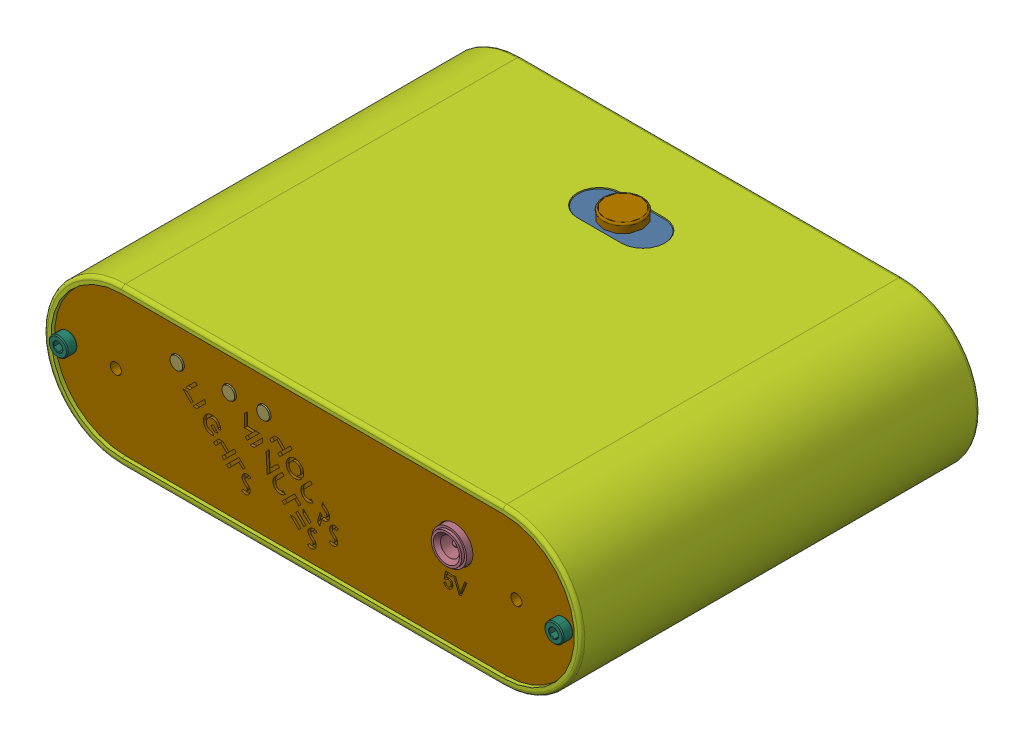
SolidWorks assembly assembly, configuration Défaut. Lengths in mm.
Overall size (155 47.3 119.91).
312 component instances, 69 part files, 68 mates.
Components (placement in the parent):
- board2-1: board2 [Défaut] at (0 -11.75 72.25) size (122.67 19.21 69.85)
  - pcb-1: pcb [Défaut] at origin size (121.6 1.5 65.9)
  - DIP18N.step-1: DIP18N.step [Défaut] at (-50.7835 3.7087 35.4382) x (0 0 1) z (-1 0 0) size (8.53 6.85 19.5)
  - DIP18N.step-2: DIP18N.step [Défaut] at (31.1067 3.7087 35.4997) x (0 0 1) z (-1 0 0) size (8.53 6.85 19.5)
  - DIP18N.step-3: DIP18N.step [Défaut] at (5.6608 3.7087 35.5611) x (0 0 1) z (-1 0 0) size (8.53 6.85 19.5)
  - DIP18N.step-4: DIP18N.step [Défaut] at (-25.3559 3.7087 35.5399) x (0 0 1) z (-1 0 0) size (8.53 6.85 19.5)
  - DIP18N.step-5: DIP18N.step [Défaut] at (-15.751 3.7087 -7.8923) x (0.008727 0 -0.999962) z (0.999962 0 0.008727) size (8.53 6.85 19.5)
  - DIP18N.step-6: DIP18N.step [Défaut] at (34.3108 3.7087 -7.8662) x (0.008727 0 -0.999962) z (0.999962 0 0.008727) size (8.53 6.85 19.5)
  - Screw Terminal Block 5mm-2: Screw Terminal Block 5mm [Valor predeterminado] at (0.4217 1.5 23.933) x (-0.999962 0 -0.008727) z (0.008727 0 -0.999962) size (10.6 16.9 9)
  - Seeeduino Xiao.step-1: Seeeduino Xiao.step [Défaut] at (-88.5187 11.44 25.9289) x (-0.008727 0 0.999962) z (-0.999962 0 -0.008727) size (17.8 4.27 22.5)
  - DS3231 RTC.step-1: DS3231 RTC.step [Défaut] at (20.896 7 25.5045) x (-1 0 0) z (0 -1 0) size (44.75 22.8 13.53)
  - zl202-8_p2-54_l10-2_w5-08_h8-89.stp-1: zl202-8_p2-54_l10-2_w5-08_h8-89.stp [Défaut] at (-55.033 1.5 3.5455) x (0 0 1) z (-1 0 0) size (10.16 11.94 5.08)
- box-1: box [Défaut] at (0 0 115) x (-1 0 0) z (0 0 -1) size (155 45 115)
- front-panel-1: front-panel [Défaut] at (0 0 10) size (150.6 40.6 3)
- back-panel-1: back-panel [Défaut] at (0 0 114) x (-1 0 0) z (0 0 -1) size (150.8 40.8 4)
- tubes-support-1: tubes-support [Défaut] at (0 0 31.6) size (147.45 40.6 8)
- beam-1: beam [Défaut] at (-60.75 -11 35) size (10.11 18.11 75.6)
- IN-12A.stp-1: IN-12A.stp [Défaut] at (-18 0 1.1) x (0 0 -1) z (-1 0 0) size (38.92 31 22.58)
  - 2.stp-1: 2.stp [Défaut] at origin size (2.7 24.17 15.83)
  - 3.stp-1: 3.stp [Défaut] at (-12.2 0 0) x (0 0 -1) z (-1 0 0) size (2 1.5 18.5)
  - 4.stp-1: 4.stp [Défaut] at (-12.2 0 0) x (0 0 1) z (-1 0 0) size (2 1.5 18.5)
  - 5.stp-1: 5.stp [Défaut] at (-12 0 0) x (0 0 -1) z (1 0 0) size (2.1 2.1 1)
  - 5.stp-2: 5.stp [Défaut] at (-10.8 0 0) x (0 0 -1) z (1 0 0) size (2.1 2.1 1)
  - 5.stp-3: 5.stp [Défaut] at (-9.6 0 0) x (0 0 -1) z (1 0 0) size (2.1 2.1 1)
  - 5.stp-4: 5.stp [Défaut] at (-8.4 0 0) x (0 0 -1) z (1 0 0) size (2.1 2.1 1)
  - 5.stp-5: 5.stp [Défaut] at (-7.2 0 0) x (0 0 -1) z (1 0 0) size (2.1 2.1 1)
  - 5.stp-6: 5.stp [Défaut] at (-6 0 0) x (0 0 -1) z (1 0 0) size (2.1 2.1 1)
  - 5.stp-7: 5.stp [Défaut] at (-4.8 0 0) x (0 0 -1) z (1 0 0) size (2.1 2.1 1)
  - 5.stp-8: 5.stp [Défaut] at (-3.6 0 0) x (0 0 -1) z (1 0 0) size (2.1 2.1 1)
  - 5.stp-9: 5.stp [Défaut] at (-2.4 0 0) x (0 0 -1) z (1 0 0) size (2.1 2.1 1)
  - 5.stp-10: 5.stp [Défaut] at (-1.2 0 0) x (0 0 -1) z (1 0 0) size (2.1 2.1 1)
  - 6.stp-1: 6.stp [Défaut] at (-11 16.1596 7.8778) x (0 -0.787778 0.61596) z (-1 0 0) size (2.1 2.1 1)
  - 7.stp-1: 7.stp [Défaut] at (-9.8 16.1596 7.8778) x (0 -0.787778 0.61596) z (-1 0 0) size (2.1 2.1 1)
  - 8.stp-1: 8.stp [Défaut] at (-8.6 16.1596 7.8778) x (0 -0.787778 0.61596) z (-1 0 0) size (2.1 2.1 1)
  - 9.stp-1: 9.stp [Défaut] at (-7.4 16.1596 7.8778) x (0 -0.787778 0.61596) z (-1 0 0) size (2.1 2.1 1)
  - 10.stp-1: 10.stp [Défaut] at (-6.2 16.1596 7.8778) x (0 -0.787778 0.61596) z (-1 0 0) size (2.1 2.1 1)
  - 11.stp-1: 11.stp [Défaut] at (-5 16.1596 7.8778) x (0 -0.787778 0.61596) z (-1 0 0) size (2.1 2.1 1)
  - 12.stp-1: 12.stp [Défaut] at (-3.8 16.1596 7.8778) x (0 -0.787778 0.61596) z (-1 0 0) size (2.1 2.1 1)
  - 13.stp-1: 13.stp [Défaut] at (-2.6 16.1596 7.8778) x (0 -0.787778 0.61596) z (-1 0 0) size (2.1 2.1 1)
  - 14.stp-1: 14.stp [Défaut] at (-1.4 16.1596 7.8778) x (0 -0.787778 0.61596) z (-1 0 0) size (2.1 2.1 1)
  - 15.stp-1: 15.stp [Défaut] at (-0.2 16.1596 7.8778) x (0 -0.787778 0.61596) z (-1 0 0) size (2.1 2.1 1)
  - 5.stp-11: 5.stp [Défaut] x (0 0 -1) z (1 0 0) size (2.1 2.1 1)
  - 5.stp-12: 5.stp [Défaut] at (-13.2 0 0) x (0 0 -1) z (1 0 0) size (2.1 2.1 1)
  - 16.stp-1: 16.stp [Défaut] at (1 16.1596 7.8778) x (0 -0.787778 0.61596) z (-1 0 0) size (2.1 2.1 1)
  - 17.stp-1: 17.stp [Défaut] at (-12.2 16.1596 7.8778) x (0 -0.787778 0.61596) z (-1 0 0) size (2.1 2.1 1)
  - 18.stp-1: 18.stp [Défaut] at (-13.2 0 0) x (0 0 -1) z (-1 0 0) size (15.83 24.17 12.28)
  - 19.stp-1: 19.stp [Défaut] x (1 0 0) z (0 1 0) size (1.51 1.46 20.68)
  - 20.stp-1: 20.stp [Défaut] at (1 0 0) size (4 22.27 2.42)
  - 21.stp-1: 21.stp [Défaut] at (-13.4 0 0) x (0 0 -1) z (-1 0 0) size (15.83 24.17 1)
  - 22.stp-1: 22.stp [Défaut] at (-14.4 0 0) x (0 0 -1) z (-1 0 0) size (15.83 27.29 2)
  - 23.stp-1: 23.stp [Défaut] x (0 0 -1) z (-1 0 0) size (21 31 33)
  - 24.stp-1: 24.stp [Défaut] x (0 0 -1) z (-1 0 0) size (1 1 15.5)
  - 24.stp-2: 24.stp [Défaut] at (0 -4.5 0) x (0 0 -1) z (-1 0 0) size (1 1 15.5)
  - 24.stp-3: 24.stp [Défaut] at (0 -8 -1.75) x (0 0 -1) z (-1 0 0) size (1 1 15.5)
  - 24.stp-4: 24.stp [Défaut] at (0 -9 -5.75) x (0 0 -1) z (-1 0 0) size (1 1 15.5)
  - 24.stp-5: 24.stp [Défaut] at (0 -8 -9.75) x (0 0 -1) z (-1 0 0) size (1 1 15.5)
  - 24.stp-6: 24.stp [Défaut] at (0 -4.5 -11.5) x (0 0 -1) z (-1 0 0) size (1 1 15.5)
  - 24.stp-7: 24.stp [Défaut] at (0 0 -11.5) x (0 0 -1) z (-1 0 0) size (1 1 15.5)
  - 24.stp-8: 24.stp [Défaut] at (0 4.5 -11.5) x (0 0 -1) z (-1 0 0) size (1 1 15.5)
  - 24.stp-9: 24.stp [Défaut] at (0 8 -9.75) x (0 0 -1) z (-1 0 0) size (1 1 15.5)
  - 24.stp-10: 24.stp [Défaut] at (0 9 -5.75) x (0 0 -1) z (-1 0 0) size (1 1 15.5)
  - 24.stp-11: 24.stp [Défaut] at (0 8 -1.75) x (0 0 -1) z (-1 0 0) size (1 1 15.5)
  - 24.stp-12: 24.stp [Défaut] at (0 4.5 0) x (0 0 -1) z (-1 0 0) size (1 1 15.5)
  - 25.stp-1: 25.stp [Défaut] at (-1.4 0 0) x (0 0 1) z (1 0 0) size (10.55 22 0.2)
  - 26.stp-1: 26.stp [Défaut] at (-2.6 0 0) x (0 0 1) z (1 0 0) size (11 22 0.2)
  - 27.stp-1: 27.stp [Défaut] at (-3.8 0 0) x (0 0 1) z (1 0 0) size (11 22 0.2)
  - 28.stp-1: 28.stp [Défaut] at (-5 0 0) x (0 0 1) z (1 0 0) size (10 22 0.2)
  - 29.stp-1: 29.stp [Défaut] at (-7.4 0 0) x (0 0 1) z (1 0 0) size (10 22 0.2)
  - 30.stp-1: 30.stp [Défaut] at (-9.6 0 0) x (0 0 -1) z (-1 0 0) size (10 22 0.2)
  - 31.stp-1: 31.stp [Défaut] at (-11 0 0) x (0 0 1) z (1 0 0) size (11 22 0.2)
  - 32.stp-1: 32.stp [Défaut] at (-12.2 0 0) x (0 0 1) z (1 0 0) size (2 22 0.2)
  - 33.stp-1: 33.stp [Défaut] at (-6 0 0) x (0 0 -1) z (-1 0 0) size (11 22 0.2)
  - 34.stp-1: 34.stp [Défaut] at (-8.6 0 0) x (0 0 1) z (1 0 0) size (10 22 0.2)
  - 1.stp-1: 1.stp [Défaut] at origin size (7.54 3.19 3.19)
  - 1-0.stp-1: 1-0.stp [Défaut] at origin size (11.99 9.11 6.32)
  - 1-1.stp-1: 1-1.stp [Défaut] at origin size (5.03 4.26 4.61)
  - 1-2.stp-1: 1-2.stp [Défaut] at origin size (8.17 8.42 6.65)
  - 1-3.stp-1: 1-3.stp [Défaut] at origin size (17.22 12.89 7.69)
  - 1-4.stp-1: 1-4.stp [Défaut] at origin size (13.11 12.81 7.39)
  - 1-5.stp-1: 1-5.stp [Défaut] at origin size (15.91 7.54 6.9)
  - 1-6.stp-1: 1-6.stp [Défaut] at origin size (10.39 4.47 4.23)
  - 1-7.stp-1: 1-7.stp [Défaut] at origin size (7.32 4.98 2.44)
  - 1-8.stp-1: 1-8.stp [Défaut] at origin size (10.29 4.36 5.63)
  - 1-9.stp-1: 1-9.stp [Défaut] at origin size (12.89 8.1 7.83)
- IN-12A.stp-2: IN-12A.stp [Défaut] at (-44 0 1.1) x (0 0 -1) z (-1 0 0) size (38.92 31 22.58)
  - 2.stp-1: 2.stp [Défaut] at origin size (2.7 24.17 15.83)
  - 3.stp-1: 3.stp [Défaut] at (-12.2 0 0) x (0 0 -1) z (-1 0 0) size (2 1.5 18.5)
  - 4.stp-1: 4.stp [Défaut] at (-12.2 0 0) x (0 0 1) z (-1 0 0) size (2 1.5 18.5)
  - 5.stp-1: 5.stp [Défaut] at (-12 0 0) x (0 0 -1) z (1 0 0) size (2.1 2.1 1)
  - 5.stp-2: 5.stp [Défaut] at (-10.8 0 0) x (0 0 -1) z (1 0 0) size (2.1 2.1 1)
  - 5.stp-3: 5.stp [Défaut] at (-9.6 0 0) x (0 0 -1) z (1 0 0) size (2.1 2.1 1)
  - 5.stp-4: 5.stp [Défaut] at (-8.4 0 0) x (0 0 -1) z (1 0 0) size (2.1 2.1 1)
  - 5.stp-5: 5.stp [Défaut] at (-7.2 0 0) x (0 0 -1) z (1 0 0) size (2.1 2.1 1)
  - 5.stp-6: 5.stp [Défaut] at (-6 0 0) x (0 0 -1) z (1 0 0) size (2.1 2.1 1)
  - 5.stp-7: 5.stp [Défaut] at (-4.8 0 0) x (0 0 -1) z (1 0 0) size (2.1 2.1 1)
  - 5.stp-8: 5.stp [Défaut] at (-3.6 0 0) x (0 0 -1) z (1 0 0) size (2.1 2.1 1)
  - 5.stp-9: 5.stp [Défaut] at (-2.4 0 0) x (0 0 -1) z (1 0 0) size (2.1 2.1 1)
  - 5.stp-10: 5.stp [Défaut] at (-1.2 0 0) x (0 0 -1) z (1 0 0) size (2.1 2.1 1)
  - 6.stp-1: 6.stp [Défaut] at (-11 16.1596 7.8778) x (0 -0.787778 0.61596) z (-1 0 0) size (2.1 2.1 1)
  - 7.stp-1: 7.stp [Défaut] at (-9.8 16.1596 7.8778) x (0 -0.787778 0.61596) z (-1 0 0) size (2.1 2.1 1)
  - 8.stp-1: 8.stp [Défaut] at (-8.6 16.1596 7.8778) x (0 -0.787778 0.61596) z (-1 0 0) size (2.1 2.1 1)
  - 9.stp-1: 9.stp [Défaut] at (-7.4 16.1596 7.8778) x (0 -0.787778 0.61596) z (-1 0 0) size (2.1 2.1 1)
  - 10.stp-1: 10.stp [Défaut] at (-6.2 16.1596 7.8778) x (0 -0.787778 0.61596) z (-1 0 0) size (2.1 2.1 1)
  - 11.stp-1: 11.stp [Défaut] at (-5 16.1596 7.8778) x (0 -0.787778 0.61596) z (-1 0 0) size (2.1 2.1 1)
  - 12.stp-1: 12.stp [Défaut] at (-3.8 16.1596 7.8778) x (0 -0.787778 0.61596) z (-1 0 0) size (2.1 2.1 1)
  - 13.stp-1: 13.stp [Défaut] at (-2.6 16.1596 7.8778) x (0 -0.787778 0.61596) z (-1 0 0) size (2.1 2.1 1)
  - 14.stp-1: 14.stp [Défaut] at (-1.4 16.1596 7.8778) x (0 -0.787778 0.61596) z (-1 0 0) size (2.1 2.1 1)
  - 15.stp-1: 15.stp [Défaut] at (-0.2 16.1596 7.8778) x (0 -0.787778 0.61596) z (-1 0 0) size (2.1 2.1 1)
  - 5.stp-11: 5.stp [Défaut] x (0 0 -1) z (1 0 0) size (2.1 2.1 1)
  - 5.stp-12: 5.stp [Défaut] at (-13.2 0 0) x (0 0 -1) z (1 0 0) size (2.1 2.1 1)
  - 16.stp-1: 16.stp [Défaut] at (1 16.1596 7.8778) x (0 -0.787778 0.61596) z (-1 0 0) size (2.1 2.1 1)
  - 17.stp-1: 17.stp [Défaut] at (-12.2 16.1596 7.8778) x (0 -0.787778 0.61596) z (-1 0 0) size (2.1 2.1 1)
  - 18.stp-1: 18.stp [Défaut] at (-13.2 0 0) x (0 0 -1) z (-1 0 0) size (15.83 24.17 12.28)
  - 19.stp-1: 19.stp [Défaut] x (1 0 0) z (0 1 0) size (1.51 1.46 20.68)
  - 20.stp-1: 20.stp [Défaut] at (1 0 0) size (4 22.27 2.42)
  - 21.stp-1: 21.stp [Défaut] at (-13.4 0 0) x (0 0 -1) z (-1 0 0) size (15.83 24.17 1)
  - 22.stp-1: 22.stp [Défaut] at (-14.4 0 0) x (0 0 -1) z (-1 0 0) size (15.83 27.29 2)
  - 23.stp-1: 23.stp [Défaut] x (0 0 -1) z (-1 0 0) size (21 31 33)
  - 24.stp-1: 24.stp [Défaut] x (0 0 -1) z (-1 0 0) size (1 1 15.5)
  - 24.stp-2: 24.stp [Défaut] at (0 -4.5 0) x (0 0 -1) z (-1 0 0) size (1 1 15.5)
  - 24.stp-3: 24.stp [Défaut] at (0 -8 -1.75) x (0 0 -1) z (-1 0 0) size (1 1 15.5)
  - 24.stp-4: 24.stp [Défaut] at (0 -9 -5.75) x (0 0 -1) z (-1 0 0) size (1 1 15.5)
  - 24.stp-5: 24.stp [Défaut] at (0 -8 -9.75) x (0 0 -1) z (-1 0 0) size (1 1 15.5)
  - 24.stp-6: 24.stp [Défaut] at (0 -4.5 -11.5) x (0 0 -1) z (-1 0 0) size (1 1 15.5)
  - 24.stp-7: 24.stp [Défaut] at (0 0 -11.5) x (0 0 -1) z (-1 0 0) size (1 1 15.5)
  - 24.stp-8: 24.stp [Défaut] at (0 4.5 -11.5) x (0 0 -1) z (-1 0 0) size (1 1 15.5)
  - 24.stp-9: 24.stp [Défaut] at (0 8 -9.75) x (0 0 -1) z (-1 0 0) size (1 1 15.5)
  - 24.stp-10: 24.stp [Défaut] at (0 9 -5.75) x (0 0 -1) z (-1 0 0) size (1 1 15.5)
  - 24.stp-11: 24.stp [Défaut] at (0 8 -1.75) x (0 0 -1) z (-1 0 0) size (1 1 15.5)
  - 24.stp-12: 24.stp [Défaut] at (0 4.5 0) x (0 0 -1) z (-1 0 0) size (1 1 15.5)
  - 25.stp-1: 25.stp [Défaut] at (-1.4 0 0) x (0 0 1) z (1 0 0) size (10.55 22 0.2)
  - 26.stp-1: 26.stp [Défaut] at (-2.6 0 0) x (0 0 1) z (1 0 0) size (11 22 0.2)
  - 27.stp-1: 27.stp [Défaut] at (-3.8 0 0) x (0 0 1) z (1 0 0) size (11 22 0.2)
  - 28.stp-1: 28.stp [Défaut] at (-5 0 0) x (0 0 1) z (1 0 0) size (10 22 0.2)
  - 29.stp-1: 29.stp [Défaut] at (-7.4 0 0) x (0 0 1) z (1 0 0) size (10 22 0.2)
  - 30.stp-1: 30.stp [Défaut] at (-9.6 0 0) x (0 0 -1) z (-1 0 0) size (10 22 0.2)
  - 31.stp-1: 31.stp [Défaut] at (-11 0 0) x (0 0 1) z (1 0 0) size (11 22 0.2)
  - 32.stp-1: 32.stp [Défaut] at (-12.2 0 0) x (0 0 1) z (1 0 0) size (2 22 0.2)
  - 33.stp-1: 33.stp [Défaut] at (-6 0 0) x (0 0 -1) z (-1 0 0) size (11 22 0.2)
  - 34.stp-1: 34.stp [Défaut] at (-8.6 0 0) x (0 0 1) z (1 0 0) size (10 22 0.2)
  - 1.stp-1: 1.stp [Défaut] at origin size (7.54 3.19 3.19)
  - 1-0.stp-1: 1-0.stp [Défaut] at origin size (11.99 9.11 6.32)
  - 1-1.stp-1: 1-1.stp [Défaut] at origin size (5.03 4.26 4.61)
  - 1-2.stp-1: 1-2.stp [Défaut] at origin size (8.17 8.42 6.65)
  - 1-3.stp-1: 1-3.stp [Défaut] at origin size (17.22 12.89 7.69)
  - 1-4.stp-1: 1-4.stp [Défaut] at origin size (13.11 12.81 7.39)
  - 1-5.stp-1: 1-5.stp [Défaut] at origin size (15.91 7.54 6.9)
  - 1-6.stp-1: 1-6.stp [Défaut] at origin size (10.39 4.47 4.23)
  - 1-7.stp-1: 1-7.stp [Défaut] at origin size (7.32 4.98 2.44)
  - 1-8.stp-1: 1-8.stp [Défaut] at origin size (10.29 4.36 5.63)
  - 1-9.stp-1: 1-9.stp [Défaut] at origin size (12.89 8.1 7.83)
- INS1.STEP-1: INS1.STEP [Défaut] at (0 6 17.6) x (-1 0 0) z (0 -1 0) size (7.01 43.17 6.51)
  - INS1-Glask_rper_01.STEP-1: INS1-Glask_rper_01.STEP [Défaut] at origin size (7.01 28.6 6.51)
  - INS1_Inlay_01.STEP-1: INS1_Inlay_01.STEP [Défaut] at (0 5.1 0) size (6 41.77 5.25)
- PinSocket_1x03_P2.54mm_Vertical.step-1: PinSocket_1x03_P2.54mm_Vertical.step [Défaut] at (2.54 6 38.6) x (0 1 0) z (0 0 -1) size (2.54 7.62 10.1)
- Pin Header 1x3 TH Pitch 2.54mm.stp-1: Pin Header 1x3 TH Pitch 2.54mm.stp [Défaut] at (-2.54 6 28.8) size (7.63 2.55 12.7)
- IN-12A.stp-3: IN-12A.stp [Défaut] at (18 0 1.1) x (0 0 -1) z (-1 0 0) size (38.92 31 22.58)
  - 2.stp-1: 2.stp [Défaut] at origin size (2.7 24.17 15.83)
  - 3.stp-1: 3.stp [Défaut] at (-12.2 0 0) x (0 0 -1) z (-1 0 0) size (2 1.5 18.5)
  - 4.stp-1: 4.stp [Défaut] at (-12.2 0 0) x (0 0 1) z (-1 0 0) size (2 1.5 18.5)
  - 5.stp-1: 5.stp [Défaut] at (-12 0 0) x (0 0 -1) z (1 0 0) size (2.1 2.1 1)
  - 5.stp-2: 5.stp [Défaut] at (-10.8 0 0) x (0 0 -1) z (1 0 0) size (2.1 2.1 1)
  - 5.stp-3: 5.stp [Défaut] at (-9.6 0 0) x (0 0 -1) z (1 0 0) size (2.1 2.1 1)
  - 5.stp-4: 5.stp [Défaut] at (-8.4 0 0) x (0 0 -1) z (1 0 0) size (2.1 2.1 1)
  - 5.stp-5: 5.stp [Défaut] at (-7.2 0 0) x (0 0 -1) z (1 0 0) size (2.1 2.1 1)
  - 5.stp-6: 5.stp [Défaut] at (-6 0 0) x (0 0 -1) z (1 0 0) size (2.1 2.1 1)
  - 5.stp-7: 5.stp [Défaut] at (-4.8 0 0) x (0 0 -1) z (1 0 0) size (2.1 2.1 1)
  - 5.stp-8: 5.stp [Défaut] at (-3.6 0 0) x (0 0 -1) z (1 0 0) size (2.1 2.1 1)
  - 5.stp-9: 5.stp [Défaut] at (-2.4 0 0) x (0 0 -1) z (1 0 0) size (2.1 2.1 1)
  - 5.stp-10: 5.stp [Défaut] at (-1.2 0 0) x (0 0 -1) z (1 0 0) size (2.1 2.1 1)
  - 6.stp-1: 6.stp [Défaut] at (-11 16.1596 7.8778) x (0 -0.787778 0.61596) z (-1 0 0) size (2.1 2.1 1)
  - 7.stp-1: 7.stp [Défaut] at (-9.8 16.1596 7.8778) x (0 -0.787778 0.61596) z (-1 0 0) size (2.1 2.1 1)
  - 8.stp-1: 8.stp [Défaut] at (-8.6 16.1596 7.8778) x (0 -0.787778 0.61596) z (-1 0 0) size (2.1 2.1 1)
  - 9.stp-1: 9.stp [Défaut] at (-7.4 16.1596 7.8778) x (0 -0.787778 0.61596) z (-1 0 0) size (2.1 2.1 1)
  - 10.stp-1: 10.stp [Défaut] at (-6.2 16.1596 7.8778) x (0 -0.787778 0.61596) z (-1 0 0) size (2.1 2.1 1)
  - 11.stp-1: 11.stp [Défaut] at (-5 16.1596 7.8778) x (0 -0.787778 0.61596) z (-1 0 0) size (2.1 2.1 1)
  - 12.stp-1: 12.stp [Défaut] at (-3.8 16.1596 7.8778) x (0 -0.787778 0.61596) z (-1 0 0) size (2.1 2.1 1)
  - 13.stp-1: 13.stp [Défaut] at (-2.6 16.1596 7.8778) x (0 -0.787778 0.61596) z (-1 0 0) size (2.1 2.1 1)
  - 14.stp-1: 14.stp [Défaut] at (-1.4 16.1596 7.8778) x (0 -0.787778 0.61596) z (-1 0 0) size (2.1 2.1 1)
  - 15.stp-1: 15.stp [Défaut] at (-0.2 16.1596 7.8778) x (0 -0.787778 0.61596) z (-1 0 0) size (2.1 2.1 1)
  - 5.stp-11: 5.stp [Défaut] x (0 0 -1) z (1 0 0) size (2.1 2.1 1)
  - 5.stp-12: 5.stp [Défaut] at (-13.2 0 0) x (0 0 -1) z (1 0 0) size (2.1 2.1 1)
  - 16.stp-1: 16.stp [Défaut] at (1 16.1596 7.8778) x (0 -0.787778 0.61596) z (-1 0 0) size (2.1 2.1 1)
  - 17.stp-1: 17.stp [Défaut] at (-12.2 16.1596 7.8778) x (0 -0.787778 0.61596) z (-1 0 0) size (2.1 2.1 1)
  - 18.stp-1: 18.stp [Défaut] at (-13.2 0 0) x (0 0 -1) z (-1 0 0) size (15.83 24.17 12.28)
  - 19.stp-1: 19.stp [Défaut] x (1 0 0) z (0 1 0) size (1.51 1.46 20.68)
  - 20.stp-1: 20.stp [Défaut] at (1 0 0) size (4 22.27 2.42)
  - 21.stp-1: 21.stp [Défaut] at (-13.4 0 0) x (0 0 -1) z (-1 0 0) size (15.83 24.17 1)
  - 22.stp-1: 22.stp [Défaut] at (-14.4 0 0) x (0 0 -1) z (-1 0 0) size (15.83 27.29 2)
  - 23.stp-1: 23.stp [Défaut] x (0 0 -1) z (-1 0 0) size (21 31 33)
  - 24.stp-1: 24.stp [Défaut] x (0 0 -1) z (-1 0 0) size (1 1 15.5)
  - 24.stp-2: 24.stp [Défaut] at (0 -4.5 0) x (0 0 -1) z (-1 0 0) size (1 1 15.5)
  - 24.stp-3: 24.stp [Défaut] at (0 -8 -1.75) x (0 0 -1) z (-1 0 0) size (1 1 15.5)
  - 24.stp-4: 24.stp [Défaut] at (0 -9 -5.75) x (0 0 -1) z (-1 0 0) size (1 1 15.5)
  - 24.stp-5: 24.stp [Défaut] at (0 -8 -9.75) x (0 0 -1) z (-1 0 0) size (1 1 15.5)
  - 24.stp-6: 24.stp [Défaut] at (0 -4.5 -11.5) x (0 0 -1) z (-1 0 0) size (1 1 15.5)
  - 24.stp-7: 24.stp [Défaut] at (0 0 -11.5) x (0 0 -1) z (-1 0 0) size (1 1 15.5)
  - 24.stp-8: 24.stp [Défaut] at (0 4.5 -11.5) x (0 0 -1) z (-1 0 0) size (1 1 15.5)
  - 24.stp-9: 24.stp [Défaut] at (0 8 -9.75) x (0 0 -1) z (-1 0 0) size (1 1 15.5)
  - 24.stp-10: 24.stp [Défaut] at (0 9 -5.75) x (0 0 -1) z (-1 0 0) size (1 1 15.5)
  - 24.stp-11: 24.stp [Défaut] at (0 8 -1.75) x (0 0 -1) z (-1 0 0) size (1 1 15.5)
  - 24.stp-12: 24.stp [Défaut] at (0 4.5 0) x (0 0 -1) z (-1 0 0) size (1 1 15.5)
  - 25.stp-1: 25.stp [Défaut] at (-1.4 0 0) x (0 0 1) z (1 0 0) size (10.55 22 0.2)
  - 26.stp-1: 26.stp [Défaut] at (-2.6 0 0) x (0 0 1) z (1 0 0) size (11 22 0.2)
  - 27.stp-1: 27.stp [Défaut] at (-3.8 0 0) x (0 0 1) z (1 0 0) size (11 22 0.2)
  - 28.stp-1: 28.stp [Défaut] at (-5 0 0) x (0 0 1) z (1 0 0) size (10 22 0.2)
  - 29.stp-1: 29.stp [Défaut] at (-7.4 0 0) x (0 0 1) z (1 0 0) size (10 22 0.2)
  - 30.stp-1: 30.stp [Défaut] at (-9.6 0 0) x (0 0 -1) z (-1 0 0) size (10 22 0.2)
  - 31.stp-1: 31.stp [Défaut] at (-11 0 0) x (0 0 1) z (1 0 0) size (11 22 0.2)
  - 32.stp-1: 32.stp [Défaut] at (-12.2 0 0) x (0 0 1) z (1 0 0) size (2 22 0.2)
  - 33.stp-1: 33.stp [Défaut] at (-6 0 0) x (0 0 -1) z (-1 0 0) size (11 22 0.2)
  - 34.stp-1: 34.stp [Défaut] at (-8.6 0 0) x (0 0 1) z (1 0 0) size (10 22 0.2)
  - 1.stp-1: 1.stp [Défaut] at origin size (7.54 3.19 3.19)
  - 1-0.stp-1: 1-0.stp [Défaut] at origin size (11.99 9.11 6.32)
  - 1-1.stp-1: 1-1.stp [Défaut] at origin size (5.03 4.26 4.61)
  - 1-2.stp-1: 1-2.stp [Défaut] at origin size (8.17 8.42 6.65)
  - 1-3.stp-1: 1-3.stp [Défaut] at origin size (17.22 12.89 7.69)
  - 1-4.stp-1: 1-4.stp [Défaut] at origin size (13.11 12.81 7.39)
  - 1-5.stp-1: 1-5.stp [Défaut] at origin size (15.91 7.54 6.9)
  - 1-6.stp-1: 1-6.stp [Défaut] at origin size (10.39 4.47 4.23)
  - 1-7.stp-1: 1-7.stp [Défaut] at origin size (7.32 4.98 2.44)
  - 1-8.stp-1: 1-8.stp [Défaut] at origin size (10.29 4.36 5.63)
  - 1-9.stp-1: 1-9.stp [Défaut] at origin size (12.89 8.1 7.83)
- IN-12A.stp-4: IN-12A.stp [Défaut] at (44 0 1.1) x (0 0 -1) z (-1 0 0) size (38.92 31 22.58)
  - 2.stp-1: 2.stp [Défaut] at origin size (2.7 24.17 15.83)
  - 3.stp-1: 3.stp [Défaut] at (-12.2 0 0) x (0 0 -1) z (-1 0 0) size (2 1.5 18.5)
  - 4.stp-1: 4.stp [Défaut] at (-12.2 0 0) x (0 0 1) z (-1 0 0) size (2 1.5 18.5)
  - 5.stp-1: 5.stp [Défaut] at (-12 0 0) x (0 0 -1) z (1 0 0) size (2.1 2.1 1)
  - 5.stp-2: 5.stp [Défaut] at (-10.8 0 0) x (0 0 -1) z (1 0 0) size (2.1 2.1 1)
  - 5.stp-3: 5.stp [Défaut] at (-9.6 0 0) x (0 0 -1) z (1 0 0) size (2.1 2.1 1)
  - 5.stp-4: 5.stp [Défaut] at (-8.4 0 0) x (0 0 -1) z (1 0 0) size (2.1 2.1 1)
  - 5.stp-5: 5.stp [Défaut] at (-7.2 0 0) x (0 0 -1) z (1 0 0) size (2.1 2.1 1)
  - 5.stp-6: 5.stp [Défaut] at (-6 0 0) x (0 0 -1) z (1 0 0) size (2.1 2.1 1)
  - 5.stp-7: 5.stp [Défaut] at (-4.8 0 0) x (0 0 -1) z (1 0 0) size (2.1 2.1 1)
  - 5.stp-8: 5.stp [Défaut] at (-3.6 0 0) x (0 0 -1) z (1 0 0) size (2.1 2.1 1)
  - 5.stp-9: 5.stp [Défaut] at (-2.4 0 0) x (0 0 -1) z (1 0 0) size (2.1 2.1 1)
  - 5.stp-10: 5.stp [Défaut] at (-1.2 0 0) x (0 0 -1) z (1 0 0) size (2.1 2.1 1)
  - 6.stp-1: 6.stp [Défaut] at (-11 16.1596 7.8778) x (0 -0.787778 0.61596) z (-1 0 0) size (2.1 2.1 1)
  - 7.stp-1: 7.stp [Défaut] at (-9.8 16.1596 7.8778) x (0 -0.787778 0.61596) z (-1 0 0) size (2.1 2.1 1)
  - 8.stp-1: 8.stp [Défaut] at (-8.6 16.1596 7.8778) x (0 -0.787778 0.61596) z (-1 0 0) size (2.1 2.1 1)
  - 9.stp-1: 9.stp [Défaut] at (-7.4 16.1596 7.8778) x (0 -0.787778 0.61596) z (-1 0 0) size (2.1 2.1 1)
  - 10.stp-1: 10.stp [Défaut] at (-6.2 16.1596 7.8778) x (0 -0.787778 0.61596) z (-1 0 0) size (2.1 2.1 1)
  - 11.stp-1: 11.stp [Défaut] at (-5 16.1596 7.8778) x (0 -0.787778 0.61596) z (-1 0 0) size (2.1 2.1 1)
  - 12.stp-1: 12.stp [Défaut] at (-3.8 16.1596 7.8778) x (0 -0.787778 0.61596) z (-1 0 0) size (2.1 2.1 1)
  - 13.stp-1: 13.stp [Défaut] at (-2.6 16.1596 7.8778) x (0 -0.787778 0.61596) z (-1 0 0) size (2.1 2.1 1)
  - 14.stp-1: 14.stp [Défaut] at (-1.4 16.1596 7.8778) x (0 -0.787778 0.61596) z (-1 0 0) size (2.1 2.1 1)
  - 15.stp-1: 15.stp [Défaut] at (-0.2 16.1596 7.8778) x (0 -0.787778 0.61596) z (-1 0 0) size (2.1 2.1 1)
  - 5.stp-11: 5.stp [Défaut] x (0 0 -1) z (1 0 0) size (2.1 2.1 1)
  - 5.stp-12: 5.stp [Défaut] at (-13.2 0 0) x (0 0 -1) z (1 0 0) size (2.1 2.1 1)
  - 16.stp-1: 16.stp [Défaut] at (1 16.1596 7.8778) x (0 -0.787778 0.61596) z (-1 0 0) size (2.1 2.1 1)
  - 17.stp-1: 17.stp [Défaut] at (-12.2 16.1596 7.8778) x (0 -0.787778 0.61596) z (-1 0 0) size (2.1 2.1 1)
  - 18.stp-1: 18.stp [Défaut] at (-13.2 0 0) x (0 0 -1) z (-1 0 0) size (15.83 24.17 12.28)
  - 19.stp-1: 19.stp [Défaut] x (1 0 0) z (0 1 0) size (1.51 1.46 20.68)
  - 20.stp-1: 20.stp [Défaut] at (1 0 0) size (4 22.27 2.42)
  - 21.stp-1: 21.stp [Défaut] at (-13.4 0 0) x (0 0 -1) z (-1 0 0) size (15.83 24.17 1)
  - 22.stp-1: 22.stp [Défaut] at (-14.4 0 0) x (0 0 -1) z (-1 0 0) size (15.83 27.29 2)
  - 23.stp-1: 23.stp [Défaut] x (0 0 -1) z (-1 0 0) size (21 31 33)
  - 24.stp-1: 24.stp [Défaut] x (0 0 -1) z (-1 0 0) size (1 1 15.5)
  - 24.stp-2: 24.stp [Défaut] at (0 -4.5 0) x (0 0 -1) z (-1 0 0) size (1 1 15.5)
  - 24.stp-3: 24.stp [Défaut] at (0 -8 -1.75) x (0 0 -1) z (-1 0 0) size (1 1 15.5)
  - 24.stp-4: 24.stp [Défaut] at (0 -9 -5.75) x (0 0 -1) z (-1 0 0) size (1 1 15.5)
  - 24.stp-5: 24.stp [Défaut] at (0 -8 -9.75) x (0 0 -1) z (-1 0 0) size (1 1 15.5)
  - 24.stp-6: 24.stp [Défaut] at (0 -4.5 -11.5) x (0 0 -1) z (-1 0 0) size (1 1 15.5)
  - 24.stp-7: 24.stp [Défaut] at (0 0 -11.5) x (0 0 -1) z (-1 0 0) size (1 1 15.5)
  - 24.stp-8: 24.stp [Défaut] at (0 4.5 -11.5) x (0 0 -1) z (-1 0 0) size (1 1 15.5)
  - 24.stp-9: 24.stp [Défaut] at (0 8 -9.75) x (0 0 -1) z (-1 0 0) size (1 1 15.5)
  - 24.stp-10: 24.stp [Défaut] at (0 9 -5.75) x (0 0 -1) z (-1 0 0) size (1 1 15.5)
  - 24.stp-11: 24.stp [Défaut] at (0 8 -1.75) x (0 0 -1) z (-1 0 0) size (1 1 15.5)
  - 24.stp-12: 24.stp [Défaut] at (0 4.5 0) x (0 0 -1) z (-1 0 0) size (1 1 15.5)
  - 25.stp-1: 25.stp [Défaut] at (-1.4 0 0) x (0 0 1) z (1 0 0) size (10.55 22 0.2)
  - 26.stp-1: 26.stp [Défaut] at (-2.6 0 0) x (0 0 1) z (1 0 0) size (11 22 0.2)
  - 27.stp-1: 27.stp [Défaut] at (-3.8 0 0) x (0 0 1) z (1 0 0) size (11 22 0.2)
  - 28.stp-1: 28.stp [Défaut] at (-5 0 0) x (0 0 1) z (1 0 0) size (10 22 0.2)
  - 29.stp-1: 29.stp [Défaut] at (-7.4 0 0) x (0 0 1) z (1 0 0) size (10 22 0.2)
  - 30.stp-1: 30.stp [Défaut] at (-9.6 0 0) x (0 0 -1) z (-1 0 0) size (10 22 0.2)
  - 31.stp-1: 31.stp [Défaut] at (-11 0 0) x (0 0 1) z (1 0 0) size (11 22 0.2)
  - 32.stp-1: 32.stp [Défaut] at (-12.2 0 0) x (0 0 1) z (1 0 0) size (2 22 0.2)
  - 33.stp-1: 33.stp [Défaut] at (-6 0 0) x (0 0 -1) z (-1 0 0) size (11 22 0.2)
  - 34.stp-1: 34.stp [Défaut] at (-8.6 0 0) x (0 0 1) z (1 0 0) size (10 22 0.2)
  - 1.stp-1: 1.stp [Défaut] at origin size (7.54 3.19 3.19)
  - 1-0.stp-1: 1-0.stp [Défaut] at origin size (11.99 9.11 6.32)
  - 1-1.stp-1: 1-1.stp [Défaut] at origin size (5.03 4.26 4.61)
  - 1-2.stp-1: 1-2.stp [Défaut] at origin size (8.17 8.42 6.65)
  - 1-3.stp-1: 1-3.stp [Défaut] at origin size (17.22 12.89 7.69)
  - 1-4.stp-1: 1-4.stp [Défaut] at origin size (13.11 12.81 7.39)
  - 1-5.stp-1: 1-5.stp [Défaut] at origin size (15.91 7.54 6.9)
  - 1-6.stp-1: 1-6.stp [Défaut] at origin size (10.39 4.47 4.23)
  - 1-7.stp-1: 1-7.stp [Défaut] at origin size (7.32 4.98 2.44)
  - 1-8.stp-1: 1-8.stp [Défaut] at origin size (10.29 4.36 5.63)
  - 1-9.stp-1: 1-9.stp [Défaut] at origin size (12.89 8.1 7.83)
- CA GRB LED 5mm-1: CA GRB LED 5mm [Default] at (-18 0 39.1) x (0 -1 0) z (1 0 0) size (5.12 34.2 5.5)
- CA GRB LED 5mm-2: CA GRB LED 5mm [Default] at (-44 0 39.1) x (0 -1 0) z (1 0 0) size (5.12 34.2 5.5)
- CA GRB LED 5mm-3: CA GRB LED 5mm [Default] at (18 0 39.1) x (0 -1 0) z (1 0 0) size (5.12 34.2 5.5)
- CA GRB LED 5mm-4: CA GRB LED 5mm [Default] at (44 0 39.1) x (0 -1 0) z (1 0 0) size (5.12 34.2 5.5)
- PinSocket_1x03_P2.54mm_Vertical.step-2: PinSocket_1x03_P2.54mm_Vertical.step [Défaut] at (2.54 -6 38.6) x (0 1 0) z (0 0 -1) size (2.54 7.62 10.1)
- Pin Header 1x3 TH Pitch 2.54mm.stp-2: Pin Header 1x3 TH Pitch 2.54mm.stp [Défaut] at (2.54 -6 28.8) x (-1 0 0) z (0 0 1) size (7.63 2.55 12.7)
- Symétrie_beam-2: Symétrie_beam [Défaut] at (60.75 -11 35) x (-1 0 0) z (0 0 -1) size (10.11 18.11 75.6)
- top-button-holder-1: top-button-holder [Défaut] at (0 10.5 35.6) size (29.96 12.5 22.6)
- Push Button WHITE-1: Push Button WHITE [Default] at (0 15.9 25.5) x (-1 0 0) z (0 0 -1) size (13 15.4 13)
- button-1: button [Défaut] at (0 20.1 26) size (24.8 5.7 12.2)
- back-buttons-holder-1: back-buttons-holder [Défaut] at (-27.5 10.4 106.5) x (0 1 0) z (0 0 1) size (15 40 5)
- 6x6 mm-1: 6x6 mm [Défaut] at (-40 10.4 110.8) x (0 1 0) z (1 0 0) size (8.15 10.4 6.02)
- 6x6 mm-2: 6x6 mm [Défaut] at (-15 10.4 110.8) x (0 1 0) z (1 0 0) size (8.15 10.4 6.02)
- 6x6 mm-3: 6x6 mm [Défaut] at (-25 10.4 110.8) x (0 1 0) z (1 0 0) size (8.15 10.4 6.02)
- dc jack-1: dc jack [Défaut] at (40 5 112.4) size (10 10 18.2)
- dc jack nut-1: dc jack nut [Défaut] at (40 5 109) x (0.931729 0.363156 0) z (0 0 1) size (14.07 11 2)
- INS1.STEP-3: INS1.STEP [Défaut] at (0 -6 17.6) x (-1 0 0) z (0 -1 0) size (7.01 43.17 6.51)
  - INS1-Glask_rper_01.STEP-1: INS1-Glask_rper_01.STEP [Défaut] at origin size (7.01 28.6 6.51)
  - INS1_Inlay_01.STEP-1: INS1_Inlay_01.STEP [Défaut] at (0 5.1 0) size (6 41.77 5.25)
- top-button-holder-2: top-button-holder [Défaut] at (0 -10.5 35.6) x (-1 0 0) z (0 0 1) size (29.96 12.5 22.6)
- M3 x 0.5mm Thread 14mm LONG SOCKET HEAD CAP SCREW.step-1: M3 x 0.5mm Thread 14mm LONG SOCKET HEAD CAP SCREW.step [Défaut] at (-71.5 0 100) x (-0.421588 0.906787 0) z (0 0 -1) size (5.5 5.5 17.01)
- M3 x 0.5mm Thread 14mm LONG SOCKET HEAD CAP SCREW.step-2: M3 x 0.5mm Thread 14mm LONG SOCKET HEAD CAP SCREW.step [Défaut] at (71.5 0 100) x (0.421588 0.906787 0) z (0 0 -1) size (5.5 5.5 17.01)
Mates (geometry in assembly coordinates):
- Coïncidente1: coincident anti-aligned: plane of box-1 through (55 0 0) normal (0 0 -1)
- Coïncidente2: coincident aligned: plane of box-1 through (0 0 115) normal (0 1 0)
- Coïncidente3: coincident anti-aligned: plane of box-1 through (0 0 115) normal (-1 0 0)
- Coïncidente5: coincident aligned: plane of board2-1 through (0 -11.75 72.25) normal (1 0 0)
- Coïncidente6: coincident anti-aligned: plane of box-1 through (55 0 10) normal (0 0 1); plane of front-panel-1 through (-55 0 10) normal (0 0 -1)
- Coïncidente7: coincident aligned: plane of front-panel-1 through (0 0 10) normal (1 0 0)
- Largeur1: width anti-aligned: plane of box-1 through (-55 -20.5 -146.4672) normal (0 1 0); plane of front-panel-1 through (55 20.5 -146.4672) normal (0 -1 0); plane of box-1 through (-55 -20.3 13) normal (0 -1 0); plane of front-panel-1 through (-55 20.3 13) normal (0 1 0)
- Coïncidente8: coincident aligned: plane of tubes-support-1 through (0 0 31.6) normal (1 0 0)
- Largeur2: width anti-aligned: plane of tubes-support-1 through (-55 20.3 35.6) normal (0 1 0); plane of box-1 through (-55 -20.3 35.6) normal (0 -1 0); plane of tubes-support-1 through (55 20.5 -146.4672) normal (0 -1 0); plane of box-1 through (-55 -20.5 -146.4672) normal (0 1 0)
- Parallèle1: parallel anti-aligned: plane of IN-12A.stp-1 through (-18 0 1.1) normal (0 0 -1)
- Coïncidente17: coincident anti-aligned: plane of IN-12A.stp-1 through (-18 0 1.1) normal (0 -1 0)
- Distance3: distance = 18 mm anti-aligned: plane of IN-12A.stp-1 through (-18 0 1.1) normal (-1 0 0)
- Distance4: distance = 6.5 mm anti-aligned: plane of IN-12A.stp-1/23.stp-1 through (-18 0 25.1) normal (0 0 1); plane of tubes-support-1 through (-55 0 31.6) normal (0 0 -1)
- Coïncidente20: coincident aligned: plane of IN-12A.stp-1/23.stp-1 through (-18 0 25.1) normal (0 0 1); plane of IN-12A.stp-2/23.stp-1 through (-44 0 25.1) normal (0 0 1)
- Coïncidente21: coincident anti-aligned: plane of IN-12A.stp-2 through (-44 0 1.1) normal (0 -1 0)
- Distance5: distance = 26 mm aligned: plane of IN-12A.stp-2 through (-44 0 1.1) normal (-1 0 0); plane of IN-12A.stp-1 through (-18 0 1.1) normal (-1 0 0)
- Distance7: distance = 8 mm anti-aligned: plane of INS1.STEP-1/INS1-Glask_rper_01.STEP-1 through (2.85 5.025 23.6) normal (0 0 1); plane of tubes-support-1 through (-55 0 31.6) normal (0 0 -1)
- Coïncidente28: coincident anti-aligned: plane of INS1.STEP-1 through (0 6 17.6) normal (-1 0 0)
- Distance9: distance = 6 mm anti-aligned: plane of INS1.STEP-1 through (0 6 17.6) normal (0 -1 0)
- Coaxiale4: concentric anti-aligned: cylinder of tubes-support-1 through (-18 0 31.6) axis (0 0 1) radius 2.6; cylinder of CA GRB LED 5mm-1 through (-18 0 39.1) axis (0 0 -1) radius 2.375
- Coïncidente29: coincident anti-aligned: plane of tubes-support-1 through (-18 0 38.1) normal (0 0 1); plane of CA GRB LED 5mm-1 through (-18 -2.75 38.1) normal (0 0 -1)
- Parallèle2: parallel aligned: plane of CA GRB LED 5mm-1 through (-18 0 39.1) normal (1 0 0)
- Coaxiale5: concentric anti-aligned: cylinder of CA GRB LED 5mm-2 through (-44 0 39.1) axis (0 0 -1) radius 2.375; cylinder of tubes-support-1 through (-44 0 31.6) axis (0 0 1) radius 2.6
- Coïncidente31: coincident anti-aligned: plane of tubes-support-1 through (-44 0 38.1) normal (0 0 1); plane of CA GRB LED 5mm-2 through (-44 -2.75 38.1) normal (0 0 -1)
- Parallèle3: parallel aligned: plane of CA GRB LED 5mm-1 through (-19.3863 -2.375 38.1) normal (0 -1 0); plane of CA GRB LED 5mm-2 through (-45.3863 -2.375 38.1) normal (0 -1 0)
- Coïncidente33: coincident anti-aligned: plane of PinSocket_1x03_P2.54mm_Vertical.step-1 through (-3.81 7.27 31.6) normal (0 0 -1); plane of Pin Header 1x3 TH Pitch 2.54mm.stp-1 through (-3.483 4.7046 31.6) normal (0 0 1)
- Coïncidente34: coincident aligned: plane of PinSocket_1x03_P2.54mm_Vertical.step-1 through (-3.81 7.27 38.6) normal (0 1 0); plane of Pin Header 1x3 TH Pitch 2.54mm.stp-1 through (-0.943 7.27 28.7734) normal (0 1 0)
- Coïncidente35: coincident aligned: plane of PinSocket_1x03_P2.54mm_Vertical.step-1 through (3.81 7.27 38.6) normal (1 0 0); plane of Pin Header 1x3 TH Pitch 2.54mm.stp-1 through (3.81 5.057 31.2742) normal (1 0 0)
- Largeur3: width aligned: plane of PinSocket_1x03_P2.54mm_Vertical.step-1 through (-3.81 7.27 38.6) normal (0 1 0); plane of PinSocket_1x03_P2.54mm_Vertical.step-1 through (3.81 4.73 38.6) normal (0 -1 0); plane of tubes-support-1 through (-3.91 4.63 31.6) normal (0 1 0); plane of tubes-support-1 through (-3.91 7.37 31.6) normal (0 -1 0)
- Largeur4: width anti-aligned: plane of PinSocket_1x03_P2.54mm_Vertical.step-1 through (3.81 7.27 38.6) normal (1 0 0); plane of PinSocket_1x03_P2.54mm_Vertical.step-1 through (-3.81 4.73 38.6) normal (-1 0 0); plane of tubes-support-1 through (3.91 7.37 31.6) normal (-1 0 0); plane of tubes-support-1 through (-3.91 7.37 31.6) normal (1 0 0)
- Coïncidente36: coincident aligned: plane of tubes-support-1 through (-55 0 31.6) normal (0 0 -1); plane of PinSocket_1x03_P2.54mm_Vertical.step-1 through (-3.81 7.27 31.6) normal (0 0 -1)
- Coïncidente37: coincident aligned: plane of back-panel-1 through (0 0 114) normal (0 1 0)
- Coïncidente38: coincident anti-aligned: plane of back-panel-1 through (0 0 114) normal (-1 0 0)
- Largeur6: width anti-aligned: plane of board2-1/pcb-1 through (0 -11.75 72.25) normal (0 -1 0); plane of beam-1 through (0 -10.25 72.25) normal (0 1 0); plane of board2-1/pcb-1 through (-58.75 -12 110.6) normal (0 1 0); plane of beam-1 through (-60.75 -10 110.6) normal (0 -1 0)
- Coïncidente40: coincident anti-aligned: plane of beam-1 through (-60.75 -11 35) normal (0 0 -1); plane of tubes-support-1 through (-60.95 -12.2 35) normal (0 0 1)
- Coaxiale10: concentric aligned: cylinder of tubes-support-1 through (-57.75 0 31.6) axis (0 0 1) radius 1.6; cylinder of beam-1 through (-57.75 0 35) axis (0 0 1) radius 1.6
- Coïncidente41: coincident anti-aligned: plane of back-panel-1 through (-60.95 2.2 110.6) normal (0 0 -1); plane of beam-1 through (-60.75 -11 110.6) normal (0 0 1)
- Coaxiale11: concentric anti-aligned: cylinder of back-panel-1 through (-57.75 0 114) axis (0 0 -1) radius 1.6; cylinder of beam-1 through (-57.75 0 35) axis (0 0 1) radius 1.6
- Coïncidente42: coincident anti-aligned: plane of box-1 through (-65.25 0 110) normal (0 0 1); plane of back-panel-1 through (55 0 110) normal (0 0 -1)
- Coïncidente44: coincident aligned: plane of buttons-holder-1 through (0 10.5 35.6) normal (1 0 0)
- Coïncidente45: coincident anti-aligned: plane of buttons-holder-1 through (6.1 12.9 23.1) normal (0 1 0); plane of Push Button WHITE-1 through (0 12.9 25.5) normal (0 -1 0)
- Largeur7: width anti-aligned: plane of Push Button WHITE-1 through (5.97 12.9 31.47) normal (1 0 0); plane of top-button-holder-1 through (-5.97 12.9 31.47) normal (-1 0 0); plane of Push Button WHITE-1 through (6.1 12.9 27) normal (-1 0 0); plane of top-button-holder-1 through (-6.1 12.9 27) normal (1 0 0)
- Largeur8: width anti-aligned: plane of top-button-holder-1 through (-5.1 12.9 19.4) normal (0 0 1); plane of Push Button WHITE-1 through (-5.1 12.9 31.6) normal (0 0 -1); plane of top-button-holder-1 through (5.97 12.9 19.53) normal (0 0 -1); plane of Push Button WHITE-1 through (5.97 12.9 31.47) normal (0 0 1)
- Parallèle4: parallel aligned: plane of buttons-holder-1 through (0 10.5 35.6) normal (0 1 0)
- Coïncidente47: coincident aligned: plane of tubes-support-1 through (-55 0 35.6) normal (0 0 1); plane of buttons-holder-1 through (-8.6 16.7 35.6) normal (0 0 1)
- Distance10: distance = 0.4 mm anti-aligned: plane of Push Button WHITE-1 through (1.725 20.1 27.225) normal (0 1 0); plane of box-1 through (55 20.5 -146.4672) normal (0 -1 0)
- Coïncidente48: coincident anti-aligned: plane of Push Button WHITE-1 through (1.725 20.1 27.225) normal (0 1 0); plane of button-1 through (-6.3 20.1 26) normal (0 -1 0)
- Largeur9: width aligned: plane of Push Button WHITE-1 through (-1.925 20.1 27.225) normal (-1 0 0); plane of Push Button WHITE-1 through (1.925 20.1 27.225) normal (1 0 0); plane of button-1 through (-3.3 16.6 32.1) normal (-1 0 0); plane of button-1 through (3.3 16.6 32.1) normal (1 0 0)
- Largeur10: width anti-aligned: plane of button-1 through (-6.3 22.3 32.1) normal (0 0 1); plane of button-1 through (-6.3 22.3 19.9) normal (0 0 -1); plane of box-1 through (6.3 -22.501 32.3) normal (0 0 -1); plane of box-1 through (6.3 -22.501 19.7) normal (0 0 1)
- Coïncidente49: coincident anti-aligned: plane of back-buttons-holder-1 through (-27.5 10.4 107.3) normal (0 0 1); plane of 6x6 mm-1 through (-38.2763 10.4 107.3) normal (0 0 -1)
- Largeur11: width anti-aligned: plane of back-buttons-holder-1 through (-43.1 13.8 107.3) normal (0 -1 0); plane of 6x6 mm-1 through (-43.1 7 107.3) normal (0 1 0); plane of back-buttons-holder-1 through (-43 13.4 110.8) normal (0 1 0); plane of 6x6 mm-1 through (-37 7.4 110.8) normal (0 -1 0)
- Largeur12: width anti-aligned: plane of back-buttons-holder-1 through (-36.9 7 107.3) normal (-1 0 0); plane of 6x6 mm-1 through (-43.1 7 107.3) normal (1 0 0); plane of back-buttons-holder-1 through (-37 13.4 110.8) normal (1 0 0); plane of 6x6 mm-1 through (-43 7.4 110.8) normal (-1 0 0)
- Coïncidente50: coincident aligned: plane of 6x6 mm-1 through (-37 7.4 110.8) normal (0 -1 0); plane of 6x6 mm-3 through (-22 7.4 110.8) normal (0 -1 0)
- Coïncidente51: coincident aligned: plane of 6x6 mm-1 through (-40 10.4 107.4) normal (0 0 -1); plane of 6x6 mm-3 through (-25 10.4 107.4) normal (0 0 -1)
- Coïncidente52: coincident aligned: plane of 6x6 mm-1 through (-40 10.4 107.4) normal (0 0 -1); plane of 6x6 mm-2 through (-15 10.4 107.4) normal (0 0 -1)
- Coïncidente53: coincident aligned: plane of 6x6 mm-1 through (-37 7.4 110.8) normal (0 -1 0); plane of 6x6 mm-2 through (-12 7.4 110.8) normal (0 -1 0)
- Largeur13: width anti-aligned: plane of 6x6 mm-2 through (-18 7.4 110.8) normal (-1 0 0); plane of back-buttons-holder-1 through (-12 13.4 110.8) normal (1 0 0); plane of 6x6 mm-2 through (-18.1 7 107.3) normal (1 0 0); plane of back-buttons-holder-1 through (-11.9 7 107.3) normal (-1 0 0)
- Largeur14: width aligned: plane of back-buttons-holder-1 through (-21.9 7 107.3) normal (-1 0 0); plane of 6x6 mm-3 through (-28.1 7 107.3) normal (1 0 0); plane of back-buttons-holder-1 through (-28 7.4 110.8) normal (-1 0 0); plane of 6x6 mm-3 through (-22 13.4 110.8) normal (1 0 0)
- Coïncidente54: coincident anti-aligned: plane of back-panel-1 through (55 0 111.5) normal (0 0 -1); plane of back-buttons-holder-1 through (-27.5 10.4 111.5) normal (0 0 1)
- Coïncidente55: coincident anti-aligned: plane of back-panel-1 through (40 5 112.4) normal (0 0 1); plane of dc jack-1 through (40 5 112.4) normal (0 0 -1)
- Coaxiale14: concentric anti-aligned: cylinder of back-panel-1 through (40 5 112.4) axis (0 0 1) radius 5.25; cylinder of dc jack-1 through (40 5 115.6) axis (0 0 -1) radius 5
- Coaxiale15: concentric anti-aligned: cylinder of dc jack-1 through (40 5 104.3) axis (0 0 1) radius 3.65; cylinder of dc jack nut-1 through (40 5 110) axis (0 0 -1) radius 3.55
- Coïncidente56: coincident anti-aligned: plane of back-panel-1 through (55 0 110) normal (0 0 -1); plane of dc jack nut-1 through (40 5 110) normal (0 0 1)
- Coaxiale17: concentric aligned: cylinder of board2-1/pcb-1 through (-56.75 -11.75 43.8) axis (0 1 0) radius 1.7; cylinder of beam-1 through (-56.75 -14 43.8) axis (0 1 0) radius 1.6
- Coaxiale18: concentric aligned: cylinder of back-panel-1 through (-15 10.4 114) axis (0 0 -1) radius 2; cylinder of 6x6 mm-2 through (-15 10.4 110.8) axis (0 0 -1) radius 1.82
- Coaxiale19: concentric aligned: cylinder of back-panel-1 through (-40 10.4 114) axis (0 0 -1) radius 2; cylinder of 6x6 mm-1 through (-40 10.4 110.8) axis (0 0 -1) radius 1.82
- Coaxiale20: concentric aligned: cylinder of back-panel-1 through (-71.5 0 114) axis (0 0 -1) radius 1.6; cylinder of M3 x 0.5mm Thread 14mm LONG SOCKET HEAD CAP SCREW.step-1 through (-71.5 0 117) axis (0 0 -1) radius 2.75
- Coïncidente57: coincident anti-aligned: plane of back-panel-1 through (55 0 114) normal (0 0 1); plane of M3 x 0.5mm Thread 14mm LONG SOCKET HEAD CAP SCREW.step-1 through (-71.5 0 114) normal (0 0 -1)
